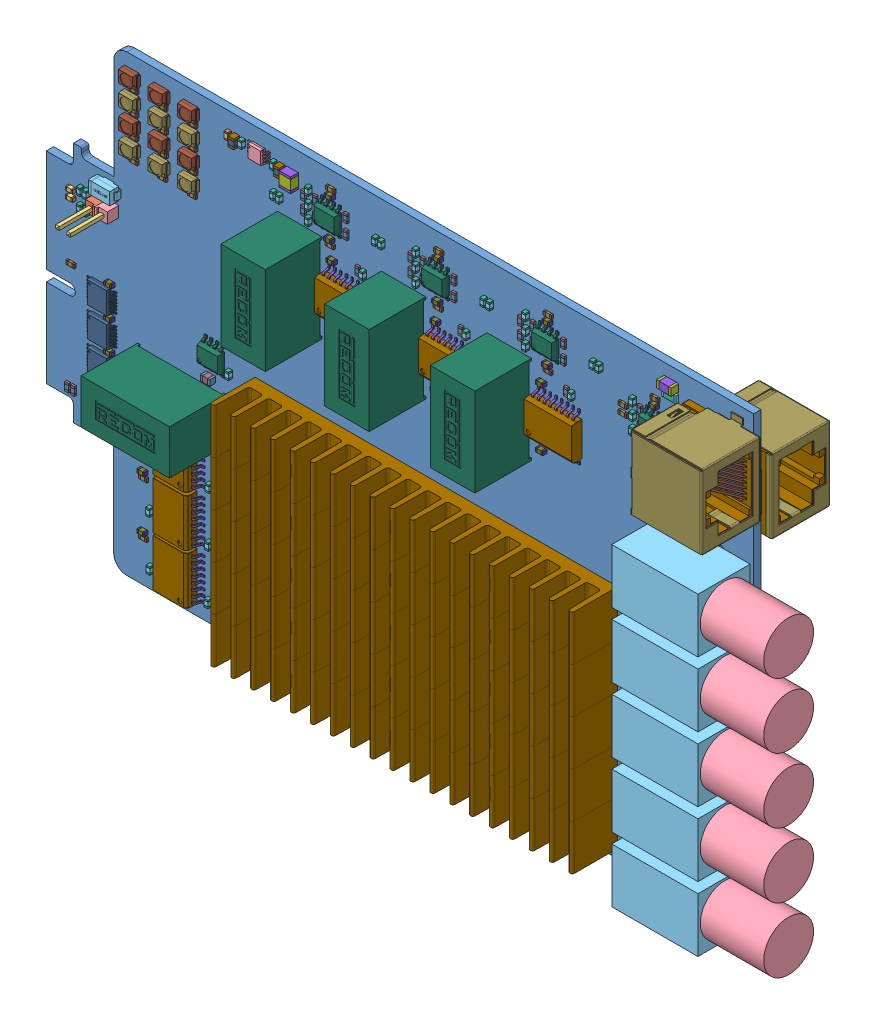
SolidWorks assembly 1166V10, configuration Standard. Lengths in mm. (continued)
Components (placement in the parent): (continued)
- 1166V10.step-1: 1166V10.step [Standard] at origin size (170.01 100 28.53) (continued)
  - D101.step-1: D101.step [Standard] at origin size (5.49 2.79 2.29)
    - DO-214AC(SMA).step-1: DO-214AC(SMA).step [Standard] at (13.8695 72.3 1.1176) x (1 0 0) z (0 -1 0) size (5.49 2.29 2.79)
  - R411.step-1: R411.step [Standard] at origin size (1.85 0.85 0.45)
    - 6547171712.step-1: 6547171712.step [Standard] at (52.85 15.2 -2.072) size (0.45 0.85 0.45)
      - Extruded-5.step-1: Extruded-5.step [Standard] at origin size (0.45 0.85 0.45)
    - 6547171712.step-2: 6547171712.step [Standard] at (51.45 15.2 -2.072) size (0.45 0.85 0.45)
      - Extruded-5.step-1: Extruded-5.step [Standard] at origin size (0.45 0.85 0.45)
    - 6547171152.step-1: 6547171152.step [Standard] at (52.15 15.2 -2.072) size (0.95 0.85 0.45)
      - Extruded-6.step-1: Extruded-6.step [Standard] at origin size (0.95 0.85 0.45)
  - R412.step-1: R412.step [Standard] at origin size (1.85 0.85 0.45)
    - 6547171712.step-1: 6547171712.step [Standard] at (50.55 12.2 -2.072) size (0.45 0.85 0.45)
      - Extruded-5.step-1: Extruded-5.step [Standard] at origin size (0.45 0.85 0.45)
    - 6547171712.step-2: 6547171712.step [Standard] at (49.15 12.2 -2.072) size (0.45 0.85 0.45)
      - Extruded-5.step-1: Extruded-5.step [Standard] at origin size (0.45 0.85 0.45)
    - 6547171152.step-1: 6547171152.step [Standard] at (49.85 12.2 -2.072) size (0.95 0.85 0.45)
      - Extruded-6.step-1: Extruded-6.step [Standard] at origin size (0.95 0.85 0.45)
  - R407.step-1: R407.step [Standard] at origin size (1.85 0.85 0.45)
    - 6547171712.step-1: 6547171712.step [Standard] at (20.25 84.8 0) size (0.45 0.85 0.45)
      - Extruded-5.step-1: Extruded-5.step [Standard] at origin size (0.45 0.85 0.45)
    - 6547171712.step-2: 6547171712.step [Standard] at (18.85 84.8 0) size (0.45 0.85 0.45)
      - Extruded-5.step-1: Extruded-5.step [Standard] at origin size (0.45 0.85 0.45)
    - 6547171152.step-1: 6547171152.step [Standard] at (19.55 84.8 0) size (0.95 0.85 0.45)
      - Extruded-6.step-1: Extruded-6.step [Standard] at origin size (0.95 0.85 0.45)
  - R405.step-1: R405.step [Standard] at origin size (1.85 0.85 0.45)
    - 6547171712.step-1: 6547171712.step [Standard] at (52.75 33.6 -2.072) size (0.45 0.85 0.45)
      - Extruded-5.step-1: Extruded-5.step [Standard] at origin size (0.45 0.85 0.45)
    - 6547171712.step-2: 6547171712.step [Standard] at (51.35 33.6 -2.072) size (0.45 0.85 0.45)
      - Extruded-5.step-1: Extruded-5.step [Standard] at origin size (0.45 0.85 0.45)
    - 6547171152.step-1: 6547171152.step [Standard] at (52.05 33.6 -2.072) size (0.95 0.85 0.45)
      - Extruded-6.step-1: Extruded-6.step [Standard] at origin size (0.95 0.85 0.45)
  - R404.step-1: R404.step [Standard] at origin size (1.85 0.85 0.45)
    - 6547171712.step-1: 6547171712.step [Standard] at (20.25 80.2 0) size (0.45 0.85 0.45)
      - Extruded-5.step-1: Extruded-5.step [Standard] at origin size (0.45 0.85 0.45)
    - 6547171712.step-2: 6547171712.step [Standard] at (18.85 80.2 0) size (0.45 0.85 0.45)
      - Extruded-5.step-1: Extruded-5.step [Standard] at origin size (0.45 0.85 0.45)
    - 6547171152.step-1: 6547171152.step [Standard] at (19.55 80.2 0) size (0.95 0.85 0.45)
      - Extruded-6.step-1: Extruded-6.step [Standard] at origin size (0.95 0.85 0.45)
  - R402.step-1: R402.step [Standard] at origin size (1.85 0.85 0.45)
    - 6547171712.step-1: 6547171712.step [Standard] at (20.25 93.8 0) size (0.45 0.85 0.45)
      - Extruded-5.step-1: Extruded-5.step [Standard] at origin size (0.45 0.85 0.45)
    - 6547171712.step-2: 6547171712.step [Standard] at (18.85 93.8 0) size (0.45 0.85 0.45)
      - Extruded-5.step-1: Extruded-5.step [Standard] at origin size (0.45 0.85 0.45)
    - 6547171152.step-1: 6547171152.step [Standard] at (19.55 93.8 0) size (0.95 0.85 0.45)
      - Extruded-6.step-1: Extruded-6.step [Standard] at origin size (0.95 0.85 0.45)
  - R406.step-1: R406.step [Standard] at origin size (1.85 0.85 0.45)
    - 6547171712.step-1: 6547171712.step [Standard] at (50.45 29.9 -2.072) size (0.45 0.85 0.45)
      - Extruded-5.step-1: Extruded-5.step [Standard] at origin size (0.45 0.85 0.45)
    - 6547171712.step-2: 6547171712.step [Standard] at (49.05 29.9 -2.072) size (0.45 0.85 0.45)
      - Extruded-5.step-1: Extruded-5.step [Standard] at origin size (0.45 0.85 0.45)
    - 6547171152.step-1: 6547171152.step [Standard] at (49.75 29.9 -2.072) size (0.95 0.85 0.45)
      - Extruded-6.step-1: Extruded-6.step [Standard] at origin size (0.95 0.85 0.45)
  - R401.step-1: R401.step [Standard] at origin size (1.85 0.85 0.45)
    - 6547171712.step-1: 6547171712.step [Standard] at (20.25 89.3 0) size (0.45 0.85 0.45)
      - Extruded-5.step-1: Extruded-5.step [Standard] at origin size (0.45 0.85 0.45)
    - 6547171712.step-2: 6547171712.step [Standard] at (18.85 89.3 0) size (0.45 0.85 0.45)
      - Extruded-5.step-1: Extruded-5.step [Standard] at origin size (0.45 0.85 0.45)
    - 6547171152.step-1: 6547171152.step [Standard] at (19.55 89.3 0) size (0.95 0.85 0.45)
      - Extruded-6.step-1: Extruded-6.step [Standard] at origin size (0.95 0.85 0.45)
  - R311.step-1: R311.step [Standard] at origin size (1.85 0.85 0.45)
    - 6547171712.step-1: 6547171712.step [Standard] at (79.85 15.2 -2.072) size (0.45 0.85 0.45)
      - Extruded-5.step-1: Extruded-5.step [Standard] at origin size (0.45 0.85 0.45)
    - 6547171712.step-2: 6547171712.step [Standard] at (78.45 15.2 -2.072) size (0.45 0.85 0.45)
      - Extruded-5.step-1: Extruded-5.step [Standard] at origin size (0.45 0.85 0.45)
    - 6547171152.step-1: 6547171152.step [Standard] at (79.15 15.2 -2.072) size (0.95 0.85 0.45)
      - Extruded-6.step-1: Extruded-6.step [Standard] at origin size (0.95 0.85 0.45)
  - R312.step-1: R312.step [Standard] at origin size (0.85 1.85 0.45)
    - 6549605008.step-1: 6549605008.step [Standard] at (78.1 11.45 -2.072) size (0.85 0.45 0.45)
      - Extruded-7.step-1: Extruded-7.step [Standard] at origin size (0.85 0.45 0.45)
    - 6549605008.step-2: 6549605008.step [Standard] at (78.1 10.05 -2.072) size (0.85 0.45 0.45)
      - Extruded-7.step-1: Extruded-7.step [Standard] at origin size (0.85 0.45 0.45)
    - 6549605488.step-1: 6549605488.step [Standard] at (78.1 10.75 -2.072) size (0.85 0.95 0.45)
      - Extruded-8.step-1: Extruded-8.step [Standard] at origin size (0.85 0.95 0.45)
  - R307.step-1: R307.step [Standard] at origin size (1.85 0.85 0.45)
    - 6547171712.step-1: 6547171712.step [Standard] at (26.75 84.8 0) size (0.45 0.85 0.45)
      - Extruded-5.step-1: Extruded-5.step [Standard] at origin size (0.45 0.85 0.45)
    - 6547171712.step-2: 6547171712.step [Standard] at (25.35 84.8 0) size (0.45 0.85 0.45)
      - Extruded-5.step-1: Extruded-5.step [Standard] at origin size (0.45 0.85 0.45)
    - 6547171152.step-1: 6547171152.step [Standard] at (26.05 84.8 0) size (0.95 0.85 0.45)
      - Extruded-6.step-1: Extruded-6.step [Standard] at origin size (0.95 0.85 0.45)
  - R305.step-1: R305.step [Standard] at origin size (1.85 0.85 0.45)
    - 6547171712.step-1: 6547171712.step [Standard] at (79.75 33.7 -2.072) size (0.45 0.85 0.45)
      - Extruded-5.step-1: Extruded-5.step [Standard] at origin size (0.45 0.85 0.45)
    - 6547171712.step-2: 6547171712.step [Standard] at (78.35 33.7 -2.072) size (0.45 0.85 0.45)
      - Extruded-5.step-1: Extruded-5.step [Standard] at origin size (0.45 0.85 0.45)
    - 6547171152.step-1: 6547171152.step [Standard] at (79.05 33.7 -2.072) size (0.95 0.85 0.45)
      - Extruded-6.step-1: Extruded-6.step [Standard] at origin size (0.95 0.85 0.45)
  - R304.step-1: R304.step [Standard] at origin size (1.85 0.85 0.45)
    - 6547171712.step-1: 6547171712.step [Standard] at (26.55 80.2 0) size (0.45 0.85 0.45)
      - Extruded-5.step-1: Extruded-5.step [Standard] at origin size (0.45 0.85 0.45)
    - 6547171712.step-2: 6547171712.step [Standard] at (25.15 80.2 0) size (0.45 0.85 0.45)
      - Extruded-5.step-1: Extruded-5.step [Standard] at origin size (0.45 0.85 0.45)
    - 6547171152.step-1: 6547171152.step [Standard] at (25.85 80.2 0) size (0.95 0.85 0.45)
      - Extruded-6.step-1: Extruded-6.step [Standard] at origin size (0.95 0.85 0.45)
  - R302.step-1: R302.step [Standard] at origin size (1.85 0.85 0.45)
    - 6547171712.step-1: 6547171712.step [Standard] at (26.65 93.8 0) size (0.45 0.85 0.45)
      - Extruded-5.step-1: Extruded-5.step [Standard] at origin size (0.45 0.85 0.45)
    - 6547171712.step-2: 6547171712.step [Standard] at (25.25 93.8 0) size (0.45 0.85 0.45)
      - Extruded-5.step-1: Extruded-5.step [Standard] at origin size (0.45 0.85 0.45)
    - 6547171152.step-1: 6547171152.step [Standard] at (25.95 93.8 0) size (0.95 0.85 0.45)
      - Extruded-6.step-1: Extruded-6.step [Standard] at origin size (0.95 0.85 0.45)
  - R306.step-1: R306.step [Standard] at origin size (1.85 0.85 0.45)
    - 6547171712.step-1: 6547171712.step [Standard] at (76.55 30.4 -2.072) size (0.45 0.85 0.45)
      - Extruded-5.step-1: Extruded-5.step [Standard] at origin size (0.45 0.85 0.45)
    - 6547171712.step-2: 6547171712.step [Standard] at (75.15 30.4 -2.072) size (0.45 0.85 0.45)
      - Extruded-5.step-1: Extruded-5.step [Standard] at origin size (0.45 0.85 0.45)
    - 6547171152.step-1: 6547171152.step [Standard] at (75.85 30.4 -2.072) size (0.95 0.85 0.45)
      - Extruded-6.step-1: Extruded-6.step [Standard] at origin size (0.95 0.85 0.45)
  - R301.step-1: R301.step [Standard] at origin size (1.85 0.85 0.45)
    - 6547171712.step-1: 6547171712.step [Standard] at (26.75 89.3 0) size (0.45 0.85 0.45)
      - Extruded-5.step-1: Extruded-5.step [Standard] at origin size (0.45 0.85 0.45)
    - 6547171712.step-2: 6547171712.step [Standard] at (25.35 89.3 0) size (0.45 0.85 0.45)
      - Extruded-5.step-1: Extruded-5.step [Standard] at origin size (0.45 0.85 0.45)
    - 6547171152.step-1: 6547171152.step [Standard] at (26.05 89.3 0) size (0.95 0.85 0.45)
      - Extruded-6.step-1: Extruded-6.step [Standard] at origin size (0.95 0.85 0.45)
  - Q402.step-1: Q402.step [Standard] at origin size (12 12 1)
    - 6545154800.step-1: 6545154800.step [Standard] at (60 14.75 -2.622) size (12 12 1)
      - Extruded-13.step-1: Extruded-13.step [Standard] at origin size (12 12 1)
  - Q401.step-1: Q401.step [Standard] at origin size (12 12 1)
    - 6545154800.step-1: 6545154800.step [Standard] at (60 33.25 -2.622) size (12 12 1)
      - Extruded-13.step-1: Extruded-13.step [Standard] at origin size (12 12 1)
  - Q302.step-1: Q302.step [Standard] at origin size (12 12 1)
    - 6545154800.step-1: 6545154800.step [Standard] at (87 14.75 -2.622) size (12 12 1)
      - Extruded-13.step-1: Extruded-13.step [Standard] at origin size (12 12 1)
  - Q301.step-1: Q301.step [Standard] at origin size (12 12 1)
    - 6545154800.step-1: 6545154800.step [Standard] at (87 33.25 -2.622) size (12 12 1)
      - Extruded-13.step-1: Extruded-13.step [Standard] at origin size (12 12 1)
  - L404.step-1: L404.step [Standard] at origin size (2 1.6 1)
    - 6545385936.step-1: 6545385936.step [Standard] at (53.275 7.1 -2.622) size (2 1.6 1)
      - Extruded-14.step-1: Extruded-14.step [Standard] at origin size (2 1.6 1)
  - L403.step-1: L403.step [Standard] at origin size (2 1.6 1)
    - 6545385936.step-1: 6545385936.step [Standard] at (53.125 25.6 -2.622) size (2 1.6 1)
      - Extruded-14.step-1: Extruded-14.step [Standard] at origin size (2 1.6 1)
  - L304.step-1: L304.step [Standard] at origin size (2 1.6 1)
    - 6545385936.step-1: 6545385936.step [Standard] at (80.375 7.1 -2.622) size (2 1.6 1)
      - Extruded-14.step-1: Extruded-14.step [Standard] at origin size (2 1.6 1)
  - L303.step-1: L303.step [Standard] at origin size (2 1.6 1)
    - 6545385936.step-1: 6545385936.step [Standard] at (80.575 25.5 -2.622) size (2 1.6 1)
      - Extruded-14.step-1: Extruded-14.step [Standard] at origin size (2 1.6 1)
  - IC403.step-1: IC403.step [Standard] at origin size (10.6 10.5 2.6)
    - SOIC-16-300.step-1: SOIC-16-300.step [Standard] at (29.6999 29.9491 1.4) x (0 -1 0) z (-1 0 0) size (10.5 2.6 10.6)
      - User_Library-SOIC-16-300_pin_SOIC_SO-300_1.step-1: User_Library-SOIC-16-300_pin_SOIC_SO-300_1.step [Standard] at (0.635 0 -3.8) x (-1 0 0) z (0 0 -1) size (0.4 1.55 1.5)
      - User_Library-SOIC-16-300_pin_SOIC_SO-300_1.step-2: User_Library-SOIC-16-300_pin_SOIC_SO-300_1.step [Standard] at (1.905 0 -3.8) x (-1 0 0) z (0 0 -1) size (0.4 1.55 1.5)
      - User_Library-SOIC-16-300_pin_SOIC_SO-300_1.step-3: User_Library-SOIC-16-300_pin_SOIC_SO-300_1.step [Standard] at (4.445 0 -3.8) x (-1 0 0) z (0 0 -1) size (0.4 1.55 1.5)
      - User_Library-SOIC-16-300_SOIC_300_SOIC_10.5X7.6_1.step-1: User_Library-SOIC-16-300_SOIC_300_SOIC_10.5X7.6_1.step [Standard] at origin size (10.5 2.35 7.6)
      - User_Library-SOIC-16-300_pin_SOIC_SO-300_1.step-4: User_Library-SOIC-16-300_pin_SOIC_SO-300_1.step [Standard] at (-3.175 0 -3.8) x (-1 0 0) z (0 0 -1) size (0.4 1.55 1.5)
      - User_Library-SOIC-16-300_pin_SOIC_SO-300_1.step-5: User_Library-SOIC-16-300_pin_SOIC_SO-300_1.step [Standard] at (-3.175 0 3.8) size (0.4 1.55 1.5)
      - User_Library-SOIC-16-300_pin_SOIC_SO-300_1.step-6: User_Library-SOIC-16-300_pin_SOIC_SO-300_1.step [Standard] at (1.905 0 3.8) size (0.4 1.55 1.5)
      - User_Library-SOIC-16-300_pin_SOIC_SO-300_1.step-7: User_Library-SOIC-16-300_pin_SOIC_SO-300_1.step [Standard] at (-1.905 0 3.8) size (0.4 1.55 1.5)
      - User_Library-SOIC-16-300_pin_SOIC_SO-300_1.step-8: User_Library-SOIC-16-300_pin_SOIC_SO-300_1.step [Standard] at (0.635 0 3.8) size (0.4 1.55 1.5)
      - User_Library-SOIC-16-300_pin_SOIC_SO-300_1.step-9: User_Library-SOIC-16-300_pin_SOIC_SO-300_1.step [Standard] at (3.175 0 3.8) size (0.4 1.55 1.5)
      - User_Library-SOIC-16-300_pin_SOIC_SO-300_1.step-10: User_Library-SOIC-16-300_pin_SOIC_SO-300_1.step [Standard] at (4.445 0 3.8) size (0.4 1.55 1.5)
      - User_Library-SOIC-16-300_pin_SOIC_SO-300_1.step-11: User_Library-SOIC-16-300_pin_SOIC_SO-300_1.step [Standard] at (-0.635 0 -3.8) x (-1 0 0) z (0 0 -1) size (0.4 1.55 1.5)
      - User_Library-SOIC-16-300_pin_SOIC_SO-300_1.step-12: User_Library-SOIC-16-300_pin_SOIC_SO-300_1.step [Standard] at (-4.445 0 3.8) size (0.4 1.55 1.5)
      - User_Library-SOIC-16-300_pin_SOIC_SO-300_1.step-13: User_Library-SOIC-16-300_pin_SOIC_SO-300_1.step [Standard] at (3.175 0 -3.8) x (-1 0 0) z (0 0 -1) size (0.4 1.55 1.5)
      - User_Library-SOIC-16-300_pin_SOIC_SO-300_1.step-14: User_Library-SOIC-16-300_pin_SOIC_SO-300_1.step [Standard] at (-0.635 0 3.8) size (0.4 1.55 1.5)
      - User_Library-SOIC-16-300_pin_SOIC_SO-300_1.step-15: User_Library-SOIC-16-300_pin_SOIC_SO-300_1.step [Standard] at (-4.445 0 -3.8) x (-1 0 0) z (0 0 -1) size (0.4 1.55 1.5)
      - User_Library-SOIC-16-300_pin_SOIC_SO-300_1.step-16: User_Library-SOIC-16-300_pin_SOIC_SO-300_1.step [Standard] at (-1.905 0 -3.8) x (-1 0 0) z (0 0 -1) size (0.4 1.55 1.5)
  - IC402.step-1: IC402.step [Standard] at origin size (10.5 10.6 2.6)
    - SOIC-16-300.step-1: SOIC-16-300.step [Standard] at (66.9491 76.6001 1.4) x (-1 0 0) z (0 1 0) size (10.5 2.6 10.6)
      - User_Library-SOIC-16-300_pin_SOIC_SO-300_1.step-1: User_Library-SOIC-16-300_pin_SOIC_SO-300_1.step [Standard] at (0.635 0 -3.8) x (-1 0 0) z (0 0 -1) size (0.4 1.55 1.5)
      - User_Library-SOIC-16-300_pin_SOIC_SO-300_1.step-2: User_Library-SOIC-16-300_pin_SOIC_SO-300_1.step [Standard] at (1.905 0 -3.8) x (-1 0 0) z (0 0 -1) size (0.4 1.55 1.5)
      - User_Library-SOIC-16-300_pin_SOIC_SO-300_1.step-3: User_Library-SOIC-16-300_pin_SOIC_SO-300_1.step [Standard] at (4.445 0 -3.8) x (-1 0 0) z (0 0 -1) size (0.4 1.55 1.5)
      - User_Library-SOIC-16-300_SOIC_300_SOIC_10.5X7.6_1.step-1: User_Library-SOIC-16-300_SOIC_300_SOIC_10.5X7.6_1.step [Standard] at origin size (10.5 2.35 7.6)
      - User_Library-SOIC-16-300_pin_SOIC_SO-300_1.step-4: User_Library-SOIC-16-300_pin_SOIC_SO-300_1.step [Standard] at (-3.175 0 -3.8) x (-1 0 0) z (0 0 -1) size (0.4 1.55 1.5)
      - User_Library-SOIC-16-300_pin_SOIC_SO-300_1.step-5: User_Library-SOIC-16-300_pin_SOIC_SO-300_1.step [Standard] at (-3.175 0 3.8) size (0.4 1.55 1.5)
      - User_Library-SOIC-16-300_pin_SOIC_SO-300_1.step-6: User_Library-SOIC-16-300_pin_SOIC_SO-300_1.step [Standard] at (1.905 0 3.8) size (0.4 1.55 1.5)
      - User_Library-SOIC-16-300_pin_SOIC_SO-300_1.step-7: User_Library-SOIC-16-300_pin_SOIC_SO-300_1.step [Standard] at (-1.905 0 3.8) size (0.4 1.55 1.5)
      - User_Library-SOIC-16-300_pin_SOIC_SO-300_1.step-8: User_Library-SOIC-16-300_pin_SOIC_SO-300_1.step [Standard] at (0.635 0 3.8) size (0.4 1.55 1.5)
      - User_Library-SOIC-16-300_pin_SOIC_SO-300_1.step-9: User_Library-SOIC-16-300_pin_SOIC_SO-300_1.step [Standard] at (3.175 0 3.8) size (0.4 1.55 1.5)
      - User_Library-SOIC-16-300_pin_SOIC_SO-300_1.step-10: User_Library-SOIC-16-300_pin_SOIC_SO-300_1.step [Standard] at (4.445 0 3.8) size (0.4 1.55 1.5)
      - User_Library-SOIC-16-300_pin_SOIC_SO-300_1.step-11: User_Library-SOIC-16-300_pin_SOIC_SO-300_1.step [Standard] at (-0.635 0 -3.8) x (-1 0 0) z (0 0 -1) size (0.4 1.55 1.5)
      - User_Library-SOIC-16-300_pin_SOIC_SO-300_1.step-12: User_Library-SOIC-16-300_pin_SOIC_SO-300_1.step [Standard] at (-4.445 0 3.8) size (0.4 1.55 1.5)
      - User_Library-SOIC-16-300_pin_SOIC_SO-300_1.step-13: User_Library-SOIC-16-300_pin_SOIC_SO-300_1.step [Standard] at (3.175 0 -3.8) x (-1 0 0) z (0 0 -1) size (0.4 1.55 1.5)
      - User_Library-SOIC-16-300_pin_SOIC_SO-300_1.step-14: User_Library-SOIC-16-300_pin_SOIC_SO-300_1.step [Standard] at (-0.635 0 3.8) size (0.4 1.55 1.5)
      - User_Library-SOIC-16-300_pin_SOIC_SO-300_1.step-15: User_Library-SOIC-16-300_pin_SOIC_SO-300_1.step [Standard] at (-4.445 0 -3.8) x (-1 0 0) z (0 0 -1) size (0.4 1.55 1.5)
      - User_Library-SOIC-16-300_pin_SOIC_SO-300_1.step-16: User_Library-SOIC-16-300_pin_SOIC_SO-300_1.step [Standard] at (-1.905 0 -3.8) x (-1 0 0) z (0 0 -1) size (0.4 1.55 1.5)
  - IC303.step-1: IC303.step [Standard] at origin size (10.6 10.5 2.6)
    - SOIC-16-300.step-1: SOIC-16-300.step [Standard] at (29.6999 18.8491 1.4) x (0 -1 0) z (-1 0 0) size (10.5 2.6 10.6)
      - User_Library-SOIC-16-300_pin_SOIC_SO-300_1.step-1: User_Library-SOIC-16-300_pin_SOIC_SO-300_1.step [Standard] at (0.635 0 -3.8) x (-1 0 0) z (0 0 -1) size (0.4 1.55 1.5)
      - User_Library-SOIC-16-300_pin_SOIC_SO-300_1.step-2: User_Library-SOIC-16-300_pin_SOIC_SO-300_1.step [Standard] at (1.905 0 -3.8) x (-1 0 0) z (0 0 -1) size (0.4 1.55 1.5)
      - User_Library-SOIC-16-300_pin_SOIC_SO-300_1.step-3: User_Library-SOIC-16-300_pin_SOIC_SO-300_1.step [Standard] at (4.445 0 -3.8) x (-1 0 0) z (0 0 -1) size (0.4 1.55 1.5)
      - User_Library-SOIC-16-300_SOIC_300_SOIC_10.5X7.6_1.step-1: User_Library-SOIC-16-300_SOIC_300_SOIC_10.5X7.6_1.step [Standard] at origin size (10.5 2.35 7.6)
      - User_Library-SOIC-16-300_pin_SOIC_SO-300_1.step-4: User_Library-SOIC-16-300_pin_SOIC_SO-300_1.step [Standard] at (-3.175 0 -3.8) x (-1 0 0) z (0 0 -1) size (0.4 1.55 1.5)
      - User_Library-SOIC-16-300_pin_SOIC_SO-300_1.step-5: User_Library-SOIC-16-300_pin_SOIC_SO-300_1.step [Standard] at (-3.175 0 3.8) size (0.4 1.55 1.5)
      - User_Library-SOIC-16-300_pin_SOIC_SO-300_1.step-6: User_Library-SOIC-16-300_pin_SOIC_SO-300_1.step [Standard] at (1.905 0 3.8) size (0.4 1.55 1.5)
      - User_Library-SOIC-16-300_pin_SOIC_SO-300_1.step-7: User_Library-SOIC-16-300_pin_SOIC_SO-300_1.step [Standard] at (-1.905 0 3.8) size (0.4 1.55 1.5)
      - User_Library-SOIC-16-300_pin_SOIC_SO-300_1.step-8: User_Library-SOIC-16-300_pin_SOIC_SO-300_1.step [Standard] at (0.635 0 3.8) size (0.4 1.55 1.5)
      - User_Library-SOIC-16-300_pin_SOIC_SO-300_1.step-9: User_Library-SOIC-16-300_pin_SOIC_SO-300_1.step [Standard] at (3.175 0 3.8) size (0.4 1.55 1.5)
      - User_Library-SOIC-16-300_pin_SOIC_SO-300_1.step-10: User_Library-SOIC-16-300_pin_SOIC_SO-300_1.step [Standard] at (4.445 0 3.8) size (0.4 1.55 1.5)
      - User_Library-SOIC-16-300_pin_SOIC_SO-300_1.step-11: User_Library-SOIC-16-300_pin_SOIC_SO-300_1.step [Standard] at (-0.635 0 -3.8) x (-1 0 0) z (0 0 -1) size (0.4 1.55 1.5)
      - User_Library-SOIC-16-300_pin_SOIC_SO-300_1.step-12: User_Library-SOIC-16-300_pin_SOIC_SO-300_1.step [Standard] at (-4.445 0 3.8) size (0.4 1.55 1.5)
      - User_Library-SOIC-16-300_pin_SOIC_SO-300_1.step-13: User_Library-SOIC-16-300_pin_SOIC_SO-300_1.step [Standard] at (3.175 0 -3.8) x (-1 0 0) z (0 0 -1) size (0.4 1.55 1.5)
      - User_Library-SOIC-16-300_pin_SOIC_SO-300_1.step-14: User_Library-SOIC-16-300_pin_SOIC_SO-300_1.step [Standard] at (-0.635 0 3.8) size (0.4 1.55 1.5)
      - User_Library-SOIC-16-300_pin_SOIC_SO-300_1.step-15: User_Library-SOIC-16-300_pin_SOIC_SO-300_1.step [Standard] at (-4.445 0 -3.8) x (-1 0 0) z (0 0 -1) size (0.4 1.55 1.5)
      - User_Library-SOIC-16-300_pin_SOIC_SO-300_1.step-16: User_Library-SOIC-16-300_pin_SOIC_SO-300_1.step [Standard] at (-1.905 0 -3.8) x (-1 0 0) z (0 0 -1) size (0.4 1.55 1.5)
  - IC302.step-1: IC302.step [Standard] at origin size (10.5 10.6 2.6)
    - SOIC-16-300.step-1: SOIC-16-300.step [Standard] at (89.8491 76.5001 1.4) x (-1 0 0) z (0 1 0) size (10.5 2.6 10.6)
      - User_Library-SOIC-16-300_pin_SOIC_SO-300_1.step-1: User_Library-SOIC-16-300_pin_SOIC_SO-300_1.step [Standard] at (0.635 0 -3.8) x (-1 0 0) z (0 0 -1) size (0.4 1.55 1.5)
      - User_Library-SOIC-16-300_pin_SOIC_SO-300_1.step-2: User_Library-SOIC-16-300_pin_SOIC_SO-300_1.step [Standard] at (1.905 0 -3.8) x (-1 0 0) z (0 0 -1) size (0.4 1.55 1.5)
      - User_Library-SOIC-16-300_pin_SOIC_SO-300_1.step-3: User_Library-SOIC-16-300_pin_SOIC_SO-300_1.step [Standard] at (4.445 0 -3.8) x (-1 0 0) z (0 0 -1) size (0.4 1.55 1.5)
      - User_Library-SOIC-16-300_SOIC_300_SOIC_10.5X7.6_1.step-1: User_Library-SOIC-16-300_SOIC_300_SOIC_10.5X7.6_1.step [Standard] at origin size (10.5 2.35 7.6)
      - User_Library-SOIC-16-300_pin_SOIC_SO-300_1.step-4: User_Library-SOIC-16-300_pin_SOIC_SO-300_1.step [Standard] at (-3.175 0 -3.8) x (-1 0 0) z (0 0 -1) size (0.4 1.55 1.5)
      - User_Library-SOIC-16-300_pin_SOIC_SO-300_1.step-5: User_Library-SOIC-16-300_pin_SOIC_SO-300_1.step [Standard] at (-3.175 0 3.8) size (0.4 1.55 1.5)
      - User_Library-SOIC-16-300_pin_SOIC_SO-300_1.step-6: User_Library-SOIC-16-300_pin_SOIC_SO-300_1.step [Standard] at (1.905 0 3.8) size (0.4 1.55 1.5)
      - User_Library-SOIC-16-300_pin_SOIC_SO-300_1.step-7: User_Library-SOIC-16-300_pin_SOIC_SO-300_1.step [Standard] at (-1.905 0 3.8) size (0.4 1.55 1.5)
      - User_Library-SOIC-16-300_pin_SOIC_SO-300_1.step-8: User_Library-SOIC-16-300_pin_SOIC_SO-300_1.step [Standard] at (0.635 0 3.8) size (0.4 1.55 1.5)
      - User_Library-SOIC-16-300_pin_SOIC_SO-300_1.step-9: User_Library-SOIC-16-300_pin_SOIC_SO-300_1.step [Standard] at (3.175 0 3.8) size (0.4 1.55 1.5)
      - User_Library-SOIC-16-300_pin_SOIC_SO-300_1.step-10: User_Library-SOIC-16-300_pin_SOIC_SO-300_1.step [Standard] at (4.445 0 3.8) size (0.4 1.55 1.5)
      - User_Library-SOIC-16-300_pin_SOIC_SO-300_1.step-11: User_Library-SOIC-16-300_pin_SOIC_SO-300_1.step [Standard] at (-0.635 0 -3.8) x (-1 0 0) z (0 0 -1) size (0.4 1.55 1.5)
      - User_Library-SOIC-16-300_pin_SOIC_SO-300_1.step-12: User_Library-SOIC-16-300_pin_SOIC_SO-300_1.step [Standard] at (-4.445 0 3.8) size (0.4 1.55 1.5)
      - User_Library-SOIC-16-300_pin_SOIC_SO-300_1.step-13: User_Library-SOIC-16-300_pin_SOIC_SO-300_1.step [Standard] at (3.175 0 -3.8) x (-1 0 0) z (0 0 -1) size (0.4 1.55 1.5)
      - User_Library-SOIC-16-300_pin_SOIC_SO-300_1.step-14: User_Library-SOIC-16-300_pin_SOIC_SO-300_1.step [Standard] at (-0.635 0 3.8) size (0.4 1.55 1.5)
      - User_Library-SOIC-16-300_pin_SOIC_SO-300_1.step-15: User_Library-SOIC-16-300_pin_SOIC_SO-300_1.step [Standard] at (-4.445 0 -3.8) x (-1 0 0) z (0 0 -1) size (0.4 1.55 1.5)
      - User_Library-SOIC-16-300_pin_SOIC_SO-300_1.step-16: User_Library-SOIC-16-300_pin_SOIC_SO-300_1.step [Standard] at (-1.905 0 -3.8) x (-1 0 0) z (0 0 -1) size (0.4 1.55 1.5)
  - IC103.step-1: IC103.step [Standard] at origin size (6.46 5 1.2)
    - TSSOP-14.step-1: TSSOP-14.step [Standard] at (12.3449 44.4441 0) x (1 0 0) z (0 -1 0) size (6.46 1.2 5)
  - IC102.step-1: IC102.step [Standard] at origin size (6.46 5 1.2)
    - TSSOP-14.step-1: TSSOP-14.step [Standard] at (12.3449 37.9441 0) x (1 0 0) z (0 -1 0) size (6.46 1.2 5)
  - D404.step-1: D404.step [Standard] at origin size (3.49 2.8 1.55)
    - PLCC2.step-1: PLCC2.step [Standard] at (18.9999 87 0.75) x (1 0 0) z (0 0 -1) size (3.49 2.8 1.55)
  - D403.step-1: D403.step [Standard] at origin size (3.53 2.81 1.55)
    - PLCC2_rot.step-1: PLCC2_rot.step [Standard] at (19 82.5 0.75) x (1 0 0) z (0 0 -1) size (3.53 2.81 1.55)
  - D402.step-1: D402.step [Standard] at origin size (3.49 2.8 1.55)
    - PLCC2.step-1: PLCC2.step [Standard] at (18.9999 96 0.75) x (1 0 0) z (0 0 -1) size (3.49 2.8 1.55)
  - D401.step-1: D401.step [Standard] at origin size (3.53 2.81 1.55)
    - PLCC2_rot.step-1: PLCC2_rot.step [Standard] at (19 91.5 0.75) x (1 0 0) z (0 0 -1) size (3.53 2.81 1.55)
  - D304.step-1: D304.step [Standard] at origin size (3.49 2.8 1.55)
    - PLCC2.step-1: PLCC2.step [Standard] at (25.4999 87 0.75) x (1 0 0) z (0 0 -1) size (3.49 2.8 1.55)
  - D303.step-1: D303.step [Standard] at origin size (3.53 2.81 1.55)
    - PLCC2_rot.step-1: PLCC2_rot.step [Standard] at (25.5 82.5 0.75) x (1 0 0) z (0 0 -1) size (3.53 2.81 1.55)
  - D302.step-1: D302.step [Standard] at origin size (3.49 2.8 1.55)
    - PLCC2.step-1: PLCC2.step [Standard] at (25.4999 96 0.75) x (1 0 0) z (0 0 -1) size (3.49 2.8 1.55)
  - D301.step-1: D301.step [Standard] at origin size (3.53 2.81 1.55)
    - PLCC2_rot.step-1: PLCC2_rot.step [Standard] at (25.5 91.5 0.75) x (1 0 0) z (0 0 -1) size (3.53 2.81 1.55)
  - CF406.step-1: CF406.step [Standard] at origin size (0.82 1.6 0.9)
    - 6547668352.step-1: 6547668352.step [Standard] at (36.3 26.35 0) size (0.82 0.9 0.9)
      - Extruded.step-1: Extruded.step [Standard] at origin size (0.82 0.9 0.9)
    - 6549602528.step-1: 6549602528.step [Standard] at (36.3 25.725 0) size (0.82 0.35 0.9)
      - Extruded-0.step-1: Extruded-0.step [Standard] at origin size (0.82 0.35 0.9)
    - 6549602528.step-2: 6549602528.step [Standard] at (36.3 26.975 0) size (0.82 0.35 0.9)
      - Extruded-0.step-1: Extruded-0.step [Standard] at origin size (0.82 0.35 0.9)
  - CF404.step-1: CF404.step [Standard] at origin size (1.6 0.82 0.9)
    - 6547664352.step-1: 6547664352.step [Standard] at (63.35 70.1 0) size (0.9 0.82 0.9)
      - Extruded-9.step-1: Extruded-9.step [Standard] at origin size (0.9 0.82 0.9)
    - 6547664912.step-1: 6547664912.step [Standard] at (62.725 70.1 0) size (0.35 0.82 0.9)
      - Extruded-10.step-1: Extruded-10.step [Standard] at origin size (0.35 0.82 0.9)
    - 6547664912.step-2: 6547664912.step [Standard] at (63.975 70.1 0) size (0.35 0.82 0.9)
      - Extruded-10.step-1: Extruded-10.step [Standard] at origin size (0.35 0.82 0.9)
  - CF306.step-1: CF306.step [Standard] at origin size (0.82 1.6 0.9)
    - 6547668352.step-1: 6547668352.step [Standard] at (36.2 15.25 0) size (0.82 0.9 0.9)
      - Extruded.step-1: Extruded.step [Standard] at origin size (0.82 0.9 0.9)
    - 6549602528.step-1: 6549602528.step [Standard] at (36.2 14.625 0) size (0.82 0.35 0.9)
      - Extruded-0.step-1: Extruded-0.step [Standard] at origin size (0.82 0.35 0.9)
    - 6549602528.step-2: 6549602528.step [Standard] at (36.2 15.875 0) size (0.82 0.35 0.9)
      - Extruded-0.step-1: Extruded-0.step [Standard] at origin size (0.82 0.35 0.9)
  - CF304.step-1: CF304.step [Standard] at origin size (1.6 0.82 0.9)
    - 6547664352.step-1: 6547664352.step [Standard] at (86.25 70 0) size (0.9 0.82 0.9)
      - Extruded-9.step-1: Extruded-9.step [Standard] at origin size (0.9 0.82 0.9)
    - 6547664912.step-1: 6547664912.step [Standard] at (85.625 70 0) size (0.35 0.82 0.9)
      - Extruded-10.step-1: Extruded-10.step [Standard] at origin size (0.35 0.82 0.9)
    - 6547664912.step-2: 6547664912.step [Standard] at (86.875 70 0) size (0.35 0.82 0.9)
      - Extruded-10.step-1: Extruded-10.step [Standard] at origin size (0.35 0.82 0.9)
  - CF103.step-1: CF103.step [Standard] at origin size (1.6 0.82 0.9)
    - 6547664912.step-1: 6547664912.step [Standard] at (13.725 41.2 0) size (0.35 0.82 0.9)
      - Extruded-10.step-1: Extruded-10.step [Standard] at origin size (0.35 0.82 0.9)
    - 6547664912.step-2: 6547664912.step [Standard] at (14.975 41.2 0) size (0.35 0.82 0.9)
      - Extruded-10.step-1: Extruded-10.step [Standard] at origin size (0.35 0.82 0.9)
    - 6547664352.step-1: 6547664352.step [Standard] at (14.35 41.2 0) size (0.9 0.82 0.9)
      - Extruded-9.step-1: Extruded-9.step [Standard] at origin size (0.9 0.82 0.9)
  - CF102.step-1: CF102.step [Standard] at origin size (1.6 0.82 0.9)
    - 6547664912.step-1: 6547664912.step [Standard] at (13.725 47.7 0) size (0.35 0.82 0.9)
      - Extruded-10.step-1: Extruded-10.step [Standard] at origin size (0.35 0.82 0.9)
    - 6547664912.step-2: 6547664912.step [Standard] at (14.975 47.7 0) size (0.35 0.82 0.9)
      - Extruded-10.step-1: Extruded-10.step [Standard] at origin size (0.35 0.82 0.9)
    - 6547664352.step-1: 6547664352.step [Standard] at (14.35 47.7 0) size (0.9 0.82 0.9)
      - Extruded-9.step-1: Extruded-9.step [Standard] at origin size (0.9 0.82 0.9)
  - C425.step-1: C425.step [Standard] at origin size (2.1 1.25 1.3)
    - 6545927808.step-1: 6545927808.step [Standard] at (57.1 7.5 -2.922) size (1.1 1.25 1.3)
      - Extruded-15.step-1: Extruded-15.step [Standard] at origin size (1.1 1.25 1.3)
    - 6545928368.step-1: 6545928368.step [Standard] at (57.9 7.5 -2.922) size (0.5 1.25 1.3)
      - Extruded-16.step-1: Extruded-16.step [Standard] at origin size (0.5 1.25 1.3)
    - 6545928368.step-2: 6545928368.step [Standard] at (56.3 7.5 -2.922) size (0.5 1.25 1.3)
      - Extruded-16.step-1: Extruded-16.step [Standard] at origin size (0.5 1.25 1.3)
  - C426.step-1: C426.step [Standard] at origin size (0.82 1.6 0.9)
    - 6547668352.step-1: 6547668352.step [Standard] at (51 11.35 -2.522) size (0.82 0.9 0.9)
      - Extruded.step-1: Extruded.step [Standard] at origin size (0.82 0.9 0.9)
    - 6549602528.step-1: 6549602528.step [Standard] at (51 11.975 -2.522) size (0.82 0.35 0.9)
      - Extruded-0.step-1: Extruded-0.step [Standard] at origin size (0.82 0.35 0.9)
    - 6549602528.step-2: 6549602528.step [Standard] at (51 10.725 -2.522) size (0.82 0.35 0.9)
      - Extruded-0.step-1: Extruded-0.step [Standard] at origin size (0.82 0.35 0.9)
  - C424.step-1: C424.step [Standard] at origin size (1.6 0.82 0.9)
    - 6547664352.step-1: 6547664352.step [Standard] at (52.15 16.4 -2.522) size (0.9 0.82 0.9)
      - Extruded-9.step-1: Extruded-9.step [Standard] at origin size (0.9 0.82 0.9)
    - 6547664912.step-1: 6547664912.step [Standard] at (52.775 16.4 -2.522) size (0.35 0.82 0.9)
      - Extruded-10.step-1: Extruded-10.step [Standard] at origin size (0.35 0.82 0.9)
    - 6547664912.step-2: 6547664912.step [Standard] at (51.525 16.4 -2.522) size (0.35 0.82 0.9)
      - Extruded-10.step-1: Extruded-10.step [Standard] at origin size (0.35 0.82 0.9)
  - C423.step-1: C423.step [Standard] at origin size (1.25 2.1 1.3)
    - 6549603008.step-1: 6549603008.step [Standard] at (52.6 10 -2.922) size (1.25 1.1 1.3)
      - Extruded-4.step-1: Extruded-4.step [Standard] at origin size (1.25 1.1 1.3)
    - 6549603568.step-1: 6549603568.step [Standard] at (52.6 10.8 -2.922) size (1.25 0.5 1.3)
      - Extruded-3.step-1: Extruded-3.step [Standard] at origin size (1.25 0.5 1.3)
    - 6549603568.step-2: 6549603568.step [Standard] at (52.6 9.2 -2.922) size (1.25 0.5 1.3)
      - Extruded-3.step-1: Extruded-3.step [Standard] at origin size (1.25 0.5 1.3)
  - C412.step-1: C412.step [Standard] at origin size (2.1 1.25 1.3)
    - 6545927808.step-1: 6545927808.step [Standard] at (57.1 25.9 -2.922) size (1.1 1.25 1.3)
      - Extruded-15.step-1: Extruded-15.step [Standard] at origin size (1.1 1.25 1.3)
    - 6545928368.step-1: 6545928368.step [Standard] at (57.9 25.9 -2.922) size (0.5 1.25 1.3)
      - Extruded-16.step-1: Extruded-16.step [Standard] at origin size (0.5 1.25 1.3)
    - 6545928368.step-2: 6545928368.step [Standard] at (56.3 25.9 -2.922) size (0.5 1.25 1.3)
      - Extruded-16.step-1: Extruded-16.step [Standard] at origin size (0.5 1.25 1.3)
  - C416.step-1: C416.step [Standard] at origin size (0.82 1.6 0.9)
    - 6547668352.step-1: 6547668352.step [Standard] at (50.9 29.05 -2.522) size (0.82 0.9 0.9)
      - Extruded.step-1: Extruded.step [Standard] at origin size (0.82 0.9 0.9)
    - 6549602528.step-1: 6549602528.step [Standard] at (50.9 29.675 -2.522) size (0.82 0.35 0.9)
      - Extruded-0.step-1: Extruded-0.step [Standard] at origin size (0.82 0.35 0.9)
    - 6549602528.step-2: 6549602528.step [Standard] at (50.9 28.425 -2.522) size (0.82 0.35 0.9)
      - Extruded-0.step-1: Extruded-0.step [Standard] at origin size (0.82 0.35 0.9)
  - C411.step-1: C411.step [Standard] at origin size (1.6 0.82 0.9)
    - 6547664352.step-1: 6547664352.step [Standard] at (52.05 34.8 -2.522) size (0.9 0.82 0.9)
      - Extruded-9.step-1: Extruded-9.step [Standard] at origin size (0.9 0.82 0.9)
    - 6547664912.step-1: 6547664912.step [Standard] at (52.675 34.8 -2.522) size (0.35 0.82 0.9)
      - Extruded-10.step-1: Extruded-10.step [Standard] at origin size (0.35 0.82 0.9)
    - 6547664912.step-2: 6547664912.step [Standard] at (51.425 34.8 -2.522) size (0.35 0.82 0.9)
      - Extruded-10.step-1: Extruded-10.step [Standard] at origin size (0.35 0.82 0.9)
  - C401.step-1: C401.step [Standard] at origin size (1.25 2.1 1.3)
    - 6549603008.step-1: 6549603008.step [Standard] at (52.5 28.5 -2.922) size (1.25 1.1 1.3)
      - Extruded-4.step-1: Extruded-4.step [Standard] at origin size (1.25 1.1 1.3)
    - 6549603568.step-1: 6549603568.step [Standard] at (52.5 29.3 -2.922) size (1.25 0.5 1.3)
      - Extruded-3.step-1: Extruded-3.step [Standard] at origin size (1.25 0.5 1.3)
    - 6549603568.step-2: 6549603568.step [Standard] at (52.5 27.7 -2.922) size (1.25 0.5 1.3)
      - Extruded-3.step-1: Extruded-3.step [Standard] at origin size (1.25 0.5 1.3)
  - C325.step-1: C325.step [Standard] at origin size (2.1 1.25 1.3)
    - 6545927808.step-1: 6545927808.step [Standard] at (84.1 7.4 -2.922) size (1.1 1.25 1.3)
      - Extruded-15.step-1: Extruded-15.step [Standard] at origin size (1.1 1.25 1.3)
    - 6545928368.step-1: 6545928368.step [Standard] at (84.9 7.4 -2.922) size (0.5 1.25 1.3)
      - Extruded-16.step-1: Extruded-16.step [Standard] at origin size (0.5 1.25 1.3)
    - 6545928368.step-2: 6545928368.step [Standard] at (83.3 7.4 -2.922) size (0.5 1.25 1.3)
      - Extruded-16.step-1: Extruded-16.step [Standard] at origin size (0.5 1.25 1.3)
  - C326.step-1: C326.step [Standard] at origin size (1.6 0.82 0.9)
    - 6547664352.step-1: 6547664352.step [Standard] at (75.95 11.6 -2.522) size (0.9 0.82 0.9)
      - Extruded-9.step-1: Extruded-9.step [Standard] at origin size (0.9 0.82 0.9)
    - 6547664912.step-1: 6547664912.step [Standard] at (76.575 11.6 -2.522) size (0.35 0.82 0.9)
      - Extruded-10.step-1: Extruded-10.step [Standard] at origin size (0.35 0.82 0.9)
    - 6547664912.step-2: 6547664912.step [Standard] at (75.325 11.6 -2.522) size (0.35 0.82 0.9)
      - Extruded-10.step-1: Extruded-10.step [Standard] at origin size (0.35 0.82 0.9)
  - C324.step-1: C324.step [Standard] at origin size (1.6 0.82 0.9)
    - 6547664352.step-1: 6547664352.step [Standard] at (79.15 16.4 -2.522) size (0.9 0.82 0.9)
      - Extruded-9.step-1: Extruded-9.step [Standard] at origin size (0.9 0.82 0.9)
    - 6547664912.step-1: 6547664912.step [Standard] at (79.775 16.4 -2.522) size (0.35 0.82 0.9)
      - Extruded-10.step-1: Extruded-10.step [Standard] at origin size (0.35 0.82 0.9)
    - 6547664912.step-2: 6547664912.step [Standard] at (78.525 16.4 -2.522) size (0.35 0.82 0.9)
      - Extruded-10.step-1: Extruded-10.step [Standard] at origin size (0.35 0.82 0.9)
  - C323.step-1: C323.step [Standard] at origin size (1.25 2.1 1.3)
    - 6549603008.step-1: 6549603008.step [Standard] at (79.7 10 -2.922) size (1.25 1.1 1.3)
      - Extruded-4.step-1: Extruded-4.step [Standard] at origin size (1.25 1.1 1.3)
    - 6549603568.step-1: 6549603568.step [Standard] at (79.7 10.8 -2.922) size (1.25 0.5 1.3)
      - Extruded-3.step-1: Extruded-3.step [Standard] at origin size (1.25 0.5 1.3)
    - 6549603568.step-2: 6549603568.step [Standard] at (79.7 9.2 -2.922) size (1.25 0.5 1.3)
      - Extruded-3.step-1: Extruded-3.step [Standard] at origin size (1.25 0.5 1.3)
  - C312.step-1: C312.step [Standard] at origin size (2.1 1.25 1.3)
    - 6545927808.step-1: 6545927808.step [Standard] at (84.1 25.9 -2.922) size (1.1 1.25 1.3)
      - Extruded-15.step-1: Extruded-15.step [Standard] at origin size (1.1 1.25 1.3)
    - 6545928368.step-1: 6545928368.step [Standard] at (84.9 25.9 -2.922) size (0.5 1.25 1.3)
      - Extruded-16.step-1: Extruded-16.step [Standard] at origin size (0.5 1.25 1.3)
    - 6545928368.step-2: 6545928368.step [Standard] at (83.3 25.9 -2.922) size (0.5 1.25 1.3)
      - Extruded-16.step-1: Extruded-16.step [Standard] at origin size (0.5 1.25 1.3)
  - C316.step-1: C316.step [Standard] at origin size (0.82 1.6 0.9)
    - 6547668352.step-1: 6547668352.step [Standard] at (78 29.55 -2.522) size (0.82 0.9 0.9)
      - Extruded.step-1: Extruded.step [Standard] at origin size (0.82 0.9 0.9)
    - 6549602528.step-1: 6549602528.step [Standard] at (78 30.175 -2.522) size (0.82 0.35 0.9)
      - Extruded-0.step-1: Extruded-0.step [Standard] at origin size (0.82 0.35 0.9)
    - 6549602528.step-2: 6549602528.step [Standard] at (78 28.925 -2.522) size (0.82 0.35 0.9)
      - Extruded-0.step-1: Extruded-0.step [Standard] at origin size (0.82 0.35 0.9)
  - C311.step-1: C311.step [Standard] at origin size (1.6 0.82 0.9)
    - 6547664352.step-1: 6547664352.step [Standard] at (79.05 34.9 -2.522) size (0.9 0.82 0.9)
      - Extruded-9.step-1: Extruded-9.step [Standard] at origin size (0.9 0.82 0.9)
    - 6547664912.step-1: 6547664912.step [Standard] at (79.675 34.9 -2.522) size (0.35 0.82 0.9)
      - Extruded-10.step-1: Extruded-10.step [Standard] at origin size (0.35 0.82 0.9)
    - 6547664912.step-2: 6547664912.step [Standard] at (78.425 34.9 -2.522) size (0.35 0.82 0.9)
      - Extruded-10.step-1: Extruded-10.step [Standard] at origin size (0.35 0.82 0.9)
  - C301.step-1: C301.step [Standard] at origin size (1.25 2.1 1.3)
    - 6549603008.step-1: 6549603008.step [Standard] at (79.6 28.5 -2.922) size (1.25 1.1 1.3)
      - Extruded-4.step-1: Extruded-4.step [Standard] at origin size (1.25 1.1 1.3)
    - 6549603568.step-1: 6549603568.step [Standard] at (79.6 29.3 -2.922) size (1.25 0.5 1.3)
      - Extruded-3.step-1: Extruded-3.step [Standard] at origin size (1.25 0.5 1.3)
    - 6549603568.step-2: 6549603568.step [Standard] at (79.6 27.7 -2.922) size (1.25 0.5 1.3)
      - Extruded-3.step-1: Extruded-3.step [Standard] at origin size (1.25 0.5 1.3)
  - R211.step-1: R211.step [Standard] at origin size (1.85 0.85 0.45)
    - 6547171152.step-1: 6547171152.step [Standard] at (106.15 15.3 -2.072) size (0.95 0.85 0.45)
      - Extruded-6.step-1: Extruded-6.step [Standard] at origin size (0.95 0.85 0.45)
    - 6547171712.step-1: 6547171712.step [Standard] at (105.45 15.3 -2.072) size (0.45 0.85 0.45)
      - Extruded-5.step-1: Extruded-5.step [Standard] at origin size (0.45 0.85 0.45)
    - 6547171712.step-2: 6547171712.step [Standard] at (106.85 15.3 -2.072) size (0.45 0.85 0.45)
      - Extruded-5.step-1: Extruded-5.step [Standard] at origin size (0.45 0.85 0.45)
  - R212.step-1: R212.step [Standard] at origin size (1.85 0.85 0.45)
    - 6547171152.step-1: 6547171152.step [Standard] at (102.95 11.5 -2.072) size (0.95 0.85 0.45)
      - Extruded-6.step-1: Extruded-6.step [Standard] at origin size (0.95 0.85 0.45)
    - 6547171712.step-1: 6547171712.step [Standard] at (102.25 11.5 -2.072) size (0.45 0.85 0.45)
      - Extruded-5.step-1: Extruded-5.step [Standard] at origin size (0.45 0.85 0.45)
    - 6547171712.step-2: 6547171712.step [Standard] at (103.65 11.5 -2.072) size (0.45 0.85 0.45)
      - Extruded-5.step-1: Extruded-5.step [Standard] at origin size (0.45 0.85 0.45)
  - R205.step-1: R205.step [Standard] at origin size (1.85 0.85 0.45)
    - 6547171152.step-1: 6547171152.step [Standard] at (106.05 33.6 -2.072) size (0.95 0.85 0.45)
      - Extruded-6.step-1: Extruded-6.step [Standard] at origin size (0.95 0.85 0.45)
    - 6547171712.step-1: 6547171712.step [Standard] at (105.35 33.6 -2.072) size (0.45 0.85 0.45)
      - Extruded-5.step-1: Extruded-5.step [Standard] at origin size (0.45 0.85 0.45)
    - 6547171712.step-2: 6547171712.step [Standard] at (106.75 33.6 -2.072) size (0.45 0.85 0.45)
      - Extruded-5.step-1: Extruded-5.step [Standard] at origin size (0.45 0.85 0.45)
  - R206.step-1: R206.step [Standard] at origin size (1.85 0.85 0.45)
    - 6547171152.step-1: 6547171152.step [Standard] at (102.95 29.9 -2.072) size (0.95 0.85 0.45)
      - Extruded-6.step-1: Extruded-6.step [Standard] at origin size (0.95 0.85 0.45)
    - 6547171712.step-1: 6547171712.step [Standard] at (102.25 29.9 -2.072) size (0.45 0.85 0.45)
      - Extruded-5.step-1: Extruded-5.step [Standard] at origin size (0.45 0.85 0.45)
    - 6547171712.step-2: 6547171712.step [Standard] at (103.65 29.9 -2.072) size (0.45 0.85 0.45)
      - Extruded-5.step-1: Extruded-5.step [Standard] at origin size (0.45 0.85 0.45)
  - R207.step-1: R207.step [Standard] at origin size (1.85 0.85 0.45)
    - 6547171712.step-1: 6547171712.step [Standard] at (33.25 84.8 0) size (0.45 0.85 0.45)
      - Extruded-5.step-1: Extruded-5.step [Standard] at origin size (0.45 0.85 0.45)
    - 6547171712.step-2: 6547171712.step [Standard] at (31.85 84.8 0) size (0.45 0.85 0.45)
      - Extruded-5.step-1: Extruded-5.step [Standard] at origin size (0.45 0.85 0.45)
    - 6547171152.step-1: 6547171152.step [Standard] at (32.55 84.8 0) size (0.95 0.85 0.45)
      - Extruded-6.step-1: Extruded-6.step [Standard] at origin size (0.95 0.85 0.45)
  - R204.step-1: R204.step [Standard] at origin size (1.85 0.85 0.45)
    - 6547171712.step-1: 6547171712.step [Standard] at (33.15 80.2 0) size (0.45 0.85 0.45)
      - Extruded-5.step-1: Extruded-5.step [Standard] at origin size (0.45 0.85 0.45)
    - 6547171712.step-2: 6547171712.step [Standard] at (31.75 80.2 0) size (0.45 0.85 0.45)
      - Extruded-5.step-1: Extruded-5.step [Standard] at origin size (0.45 0.85 0.45)
